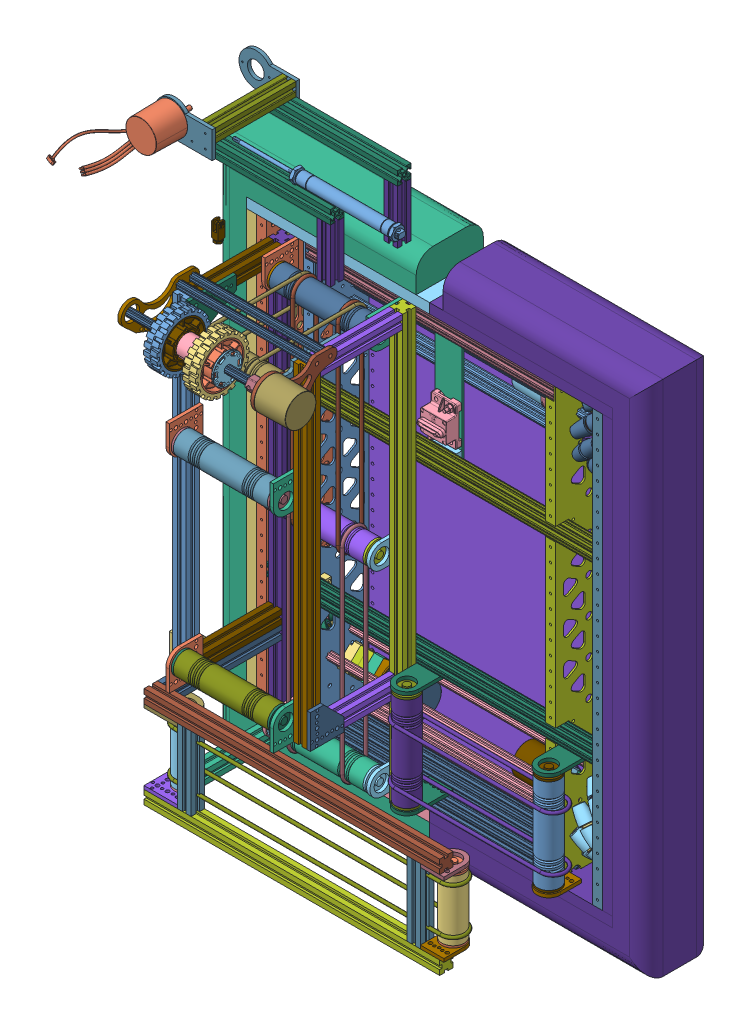
SolidWorks assembly Robot 2020, configuration Default. Lengths in mm. (continued)
Components (placement in the parent): (continued)
- Robot 2020(2)^Robot 2020-1: Robot 2020(2)^Robot 2020 [Default] at origin size (819.15 992.53 549) (virtual) (continued)
  - Snake^Robot 2020(2)_Robot 2020-1: Snake^Robot 2020(2)_Robot 2020 [Default] at (-279.4 -406.4 122.2875) x (0 -1 0) z (0 0 1) size (812.8 266.7 245.82) (virtual) (continued)
    - Longest Belt^Snake_Robot 2020(2)_Robot 2020-2: Longest Belt^Snake_Robot 2020(2)_Robot 2020 [Default] at (-411.1625 176.276 39.6875) size (421.79 6 50.31) (virtual)
    - Front Bearing Bracket^Snake_Robot 2020(2)_Robot 2020-1: Front Bearing Bracket^Snake_Robot 2020(2)_Robot 2020 [Default] at (-812.8 222.25 180.975) size (63.5 6.35 127) (virtual)
    - Front Bearing Bracket_1^Snake_Robot 2020(2)_Robot 2020-1: Front Bearing Bracket_1^Snake_Robot 2020(2)_Robot 2020 [Default] at (-812.8 25.4 180.975) size (63.5 6.35 127) (virtual)
  - Serializer^Robot 2020(2)_Robot 2020-1: Serializer^Robot 2020(2)_Robot 2020 [Default] at (-279.4 -406.4 96.8875) size (577.61 228.6 285.75) (virtual)
    - Roller_6^Serializer_Robot 2020(2)_Robot 2020-1: Roller_6^Serializer_Robot 2020(2)_Robot 2020 [Default] at origin size (42.07 200.15 42.07) (virtual)
      - Roller Hub^Roller_6_Serializer_Robot 2020(2)_Robot 2020-1: Roller Hub^Roller_6_Serializer_Robot 2020(2)_Robot 2020 [Default] at (276.225 31.75 65.0875) size (42.07 25.4 42.07) (virtual)
      - Roller 7^Roller_6_Serializer_Robot 2020(2)_Robot 2020-1: Roller 7^Roller_6_Serializer_Robot 2020(2)_Robot 2020 [Default] at (276.225 125.476 65.0875) size (42.07 177.8 42.07) (virtual)
      - Roller Hub^Roller_6_Serializer_Robot 2020(2)_Robot 2020-2: Roller Hub^Roller_6_Serializer_Robot 2020(2)_Robot 2020 [Default] at (276.225 219.202 65.0875) x (1 0 0) z (0 0 -1) size (42.07 25.4 42.07) (virtual)
    - Roller_7^Serializer_Robot 2020(2)_Robot 2020-1: Roller_7^Serializer_Robot 2020(2)_Robot 2020 [Default] at origin size (42.07 200.15 42.07) (virtual)
      - Roller Hub^Roller_7_Serializer_Robot 2020(2)_Robot 2020-1: Roller Hub^Roller_7_Serializer_Robot 2020(2)_Robot 2020 [Default] at (544.5125 31.75 65.0875) size (42.07 25.4 42.07) (virtual)
      - Roller 7^Roller_7_Serializer_Robot 2020(2)_Robot 2020-1: Roller 7^Roller_7_Serializer_Robot 2020(2)_Robot 2020 [Default] at (544.5125 125.476 65.0875) size (42.07 177.8 42.07) (virtual)
      - Roller Hub^Roller_7_Serializer_Robot 2020(2)_Robot 2020-2: Roller Hub^Roller_7_Serializer_Robot 2020(2)_Robot 2020 [Default] at (544.5125 219.202 65.0875) x (1 0 0) z (0 0 -1) size (42.07 25.4 42.07) (virtual)
    - Roller Short^Serializer_Robot 2020(2)_Robot 2020-1: Roller Short^Serializer_Robot 2020(2)_Robot 2020 [Default] at origin size (42.07 136.65 42.07) (virtual)
      - Roller Hub^Roller Short_Serializer_Robot 2020(2)_Robot 2020-1: Roller Hub^Roller Short_Serializer_Robot 2020(2)_Robot 2020 [Default] at (544.5125 31.75 246.0625) size (42.07 25.4 42.07) (virtual)
      - Roller 4.5^Roller Short_Serializer_Robot 2020(2)_Robot 2020-1: Roller 4.5^Roller Short_Serializer_Robot 2020(2)_Robot 2020 [Default] at (544.5125 93.726 246.0625) size (42.07 114.3 42.07) (virtual)
      - Roller Hub^Roller Short_Serializer_Robot 2020(2)_Robot 2020-2: Roller Hub^Roller Short_Serializer_Robot 2020(2)_Robot 2020 [Default] at (544.5125 155.702 246.0625) x (1 0 0) z (0 0 -1) size (42.07 25.4 42.07) (virtual)
    - Roller Short_1^Serializer_Robot 2020(2)_Robot 2020-1: Roller Short_1^Serializer_Robot 2020(2)_Robot 2020 [Default] at origin size (42.07 136.65 42.07) (virtual)
      - Roller Hub^Roller Short_1_Serializer_Robot 2020(2)_Robot 2020-1: Roller Hub^Roller Short_1_Serializer_Robot 2020(2)_Robot 2020 [Default] at (39.6875 31.75 246.0625) size (42.07 25.4 42.07) (virtual)
      - Roller 4.5^Roller Short_1_Serializer_Robot 2020(2)_Robot 2020-1: Roller 4.5^Roller Short_1_Serializer_Robot 2020(2)_Robot 2020 [Default] at (39.6875 93.726 246.0625) size (42.07 114.3 42.07) (virtual)
      - Roller Hub^Roller Short_1_Serializer_Robot 2020(2)_Robot 2020-2: Roller Hub^Roller Short_1_Serializer_Robot 2020(2)_Robot 2020 [Default] at (39.6875 155.702 246.0625) x (1 0 0) z (0 0 -1) size (42.07 25.4 42.07) (virtual)
    - 1010-8.25^Serializer_Robot 2020(2)_Robot 2020-1: 1010-8.25^Serializer_Robot 2020(2)_Robot 2020 [Default] at (12.7 12.7 50.8) size (25.4 25.4 209.55) (virtual)
    - 1010-22^Serializer_Robot 2020(2)_Robot 2020-1: 1010-22^Serializer_Robot 2020(2)_Robot 2020 [Default] at (0 12.7 273.05) x (0 0 -1) z (1 0 0) size (25.4 25.4 558.8) (virtual)
    - Corner Bearing Bracket^Serializer_Robot 2020(2)_Robot 2020-1: Corner Bearing Bracket^Serializer_Robot 2020(2)_Robot 2020 [Default] at (0 25.4 285.75) x (0 0 -1) z (1 0 0) size (63.5 6.35 63.5) (virtual)
    - Center Bearing Bracket^Serializer_Robot 2020(2)_Robot 2020-1: Center Bearing Bracket^Serializer_Robot 2020(2)_Robot 2020 [Default] at (522.2875 25.4 25.4) size (44.45 6.35 61.91) (virtual)
    - Center Bearing Bracket^Serializer_Robot 2020(2)_Robot 2020-2: Center Bearing Bracket^Serializer_Robot 2020(2)_Robot 2020 [Default] at (566.7375 25.4 285.75) x (-1 0 0) z (0 0 -1) size (44.45 6.35 61.91) (virtual)
    - 1010-8.25 v1(Mirror)^Serializer_Robot 2020(2)_Robot 2020-1: 1010-8.25 v1(Mirror)^Serializer_Robot 2020(2)_Robot 2020 [Default] at (12.7 177.8 50.8) x (1 0 0) z (0 0 -1) size (25.4 25.4 209.55) (virtual)
    - 1010-22 v1(Mirror)^Serializer_Robot 2020(2)_Robot 2020-1: 1010-22 v1(Mirror)^Serializer_Robot 2020(2)_Robot 2020 [Default] at (0 177.8 273.05) x (0 0 -1) z (-1 0 0) size (25.4 25.4 558.8) (virtual)
    - Corner Bearing Bracket v2(Mirror)^Serializer_Robot 2020(2)_Robot 2020-1: Corner Bearing Bracket v2(Mirror)^Serializer_Robot 2020(2)_Robot 2020 [Default] at (0 165.1 285.75) x (0 0 -1) z (-1 0 0) size (63.5 6.35 63.5) (virtual)
    - Center Bearing Bracket v3(Mirror)^Serializer_Robot 2020(2)_Robot 2020-1: Center Bearing Bracket v3(Mirror)^Serializer_Robot 2020(2)_Robot 2020 [Default] at (566.7375 165.1 285.75) x (-1 0 0) z (0 0 1) size (44.45 6.35 61.91) (virtual)
    - 1010-5.5^Serializer_Robot 2020(2)_Robot 2020-1: 1010-5.5^Serializer_Robot 2020(2)_Robot 2020 [Default] at (76.2 25.4 273.05) x (1 0 0) z (0 1 0) size (25.4 25.4 139.7) (virtual)
    - 1010-5.5^Serializer_Robot 2020(2)_Robot 2020-2: 1010-5.5^Serializer_Robot 2020(2)_Robot 2020 [Default] at (509.5875 165.1 273.05) x (1 0 0) z (0 -1 0) size (25.4 25.4 139.7) (virtual)
    - Center Bearing Bracket Tall^Serializer_Robot 2020(2)_Robot 2020-1: Center Bearing Bracket Tall^Serializer_Robot 2020(2)_Robot 2020 [Default] at (254 222.25 0) size (44.45 6.35 87.31) (virtual)
    - Center Bearing Bracket Tall^Serializer_Robot 2020(2)_Robot 2020-2: Center Bearing Bracket Tall^Serializer_Robot 2020(2)_Robot 2020 [Default] at (522.2875 222.25 0) size (44.45 6.35 87.31) (virtual)
    - Center Bearing Bracket Tall^Serializer_Robot 2020(2)_Robot 2020-3: Center Bearing Bracket Tall^Serializer_Robot 2020(2)_Robot 2020 [Default] at (254 25.4 0) size (44.45 6.35 87.31) (virtual)
    - Serializer Long Belt^Serializer_Robot 2020(2)_Robot 2020-1: Serializer Long Belt^Serializer_Robot 2020(2)_Robot 2020 [Default] at (39.6875 50.926 246.0625) size (555.14 6 50.31) (virtual)
    - Serializer Long Belt^Serializer_Robot 2020(2)_Robot 2020-2: Serializer Long Belt^Serializer_Robot 2020(2)_Robot 2020 [Default] at (39.6875 136.526 246.0625) size (555.14 6 50.31) (virtual)
    - Serializer Short Belt^Serializer_Robot 2020(2)_Robot 2020-1: Serializer Short Belt^Serializer_Robot 2020(2)_Robot 2020 [Default] at (276.225 66.676 65.0875) size (326.54 6 50.31) (virtual)
    - Serializer Short Belt^Serializer_Robot 2020(2)_Robot 2020-2: Serializer Short Belt^Serializer_Robot 2020(2)_Robot 2020 [Default] at (276.225 168.276 65.0875) size (326.54 6 50.31) (virtual)
  - Shooter Assembly^Robot 2020(2)_Robot 2020-1: Shooter Assembly^Robot 2020(2)_Robot 2020 [Default] at (-152.4 406.3995 328.6625) x (0 -1 0) z (0 0 1) size (189.59 325.45 222.03) (virtual)
    - Wheel Assembly^Shooter Assembly_Robot 2020(2)_Robot 2020-1: Wheel Assembly^Shooter Assembly_Robot 2020(2)_Robot 2020 [Default] at (-2.4561 -5.69 76.4329) x (0.5 0 0.866025) z (0 -1 0) size (138.79 138.79 119.38) (virtual)
      - am-2256 HiGrip Wheel-1: am-2256 HiGrip Wheel [Default] at (-0.933 3.4526 44.5642) x (0 0 1) z (0.866025 -0.5 0) size (35.12 101.6 101.6)
        - 4in 2013 Hub^am-2256 HiGrip Wheel-1: 4in 2013 Hub^am-2256 HiGrip Wheel [Default] at (-8.0517 2.5236 2.5343) size (35.12 82.55 82.55) (virtual)
        - 4 in tread^am-2256 HiGrip Wheel-1: 4 in tread^am-2256 HiGrip Wheel [Default] at (-8.0517 2.5236 2.5343) size (25.4 101.6 101.6) (virtual)
      - am-2256 4 in HiGrip Wheel_1^Wheel Assembly_Shooter Assembly_Robot 2020(2)_Robot 2020-1: am-2256 4 in HiGrip Wheel_1^Wheel Assembly_Shooter Assembly_Robot 2020(2)_Robot 2020 [Default] at (-3.4565 0.9183 -28.4608) x (0 0 1) z (0.866025 0.5 0) size (35.12 101.6 101.6) (virtual)
        - 4in 2013 Hub^am-2256 4 in HiGrip Wheel_1_Wheel Assembly_Shooter Assembly_Robot 2020(2)_Robot 2020-1: 4in 2013 Hub^am-2256 4 in HiGrip Wheel_1_Wheel Assembly_Shooter Assembly_Robot 2020(2)_Robot 2020 [Default] at (-8.0517 2.5236 2.5343) size (35.12 82.55 82.55) (virtual)
        - 4 in tread^am-2256 4 in HiGrip Wheel_1_Wheel Assembly_Shooter Assembly_Robot 2020(2)_Robot 2020-1: 4 in tread^am-2256 4 in HiGrip Wheel_1_Wheel Assembly_Shooter Assembly_Robot 2020(2)_Robot 2020 [Default] at (-8.0517 2.5236 2.5343) size (25.4 101.6 101.6) (virtual)
      - Wheel Center Spacer^Wheel Assembly_Shooter Assembly_Robot 2020(2)_Robot 2020-1: Wheel Center Spacer^Wheel Assembly_Shooter Assembly_Robot 2020(2)_Robot 2020 [Default] at origin size (37.36 38.1 50.8) (virtual)
      - 1_2_Hex_Bore_Aluminum_Versa Hub-1: 1_2_Hex_Bore_Aluminum_Versa Hub [Default] at (0 0 -46.99) x (0 0 -1) z (0.866025 0.5 0) size (12.7 55.88 55.88)
      - 1_2_Hex_Bore_Aluminum_VersaHub_217-2592 v1(Mirror)_1^Wheel Assembly_Shooter Assembly_Robot 2020(2)_Robot 2020-1: 1_2_Hex_Bore_Aluminum_VersaHub_217-2592 v1(Mirror)_1^Wheel Assembly_Shooter Assembly_Robot 2020(2)_Robot 2020 [Default] at (0 0 46.99) x (0 0 1) z (-0.866025 -0.5 0) size (12.7 55.88 55.88) (virtual)
    - Frame Bottom Pivot^Shooter Assembly_Robot 2020(2)_Robot 2020-1: Frame Bottom Pivot^Shooter Assembly_Robot 2020(2)_Robot 2020 [Default] at (57.6875 -114.3 11.2014) size (49 22.4 25.4) (virtual)
    - Frame Bottom Pivot v1(Mirror)^Shooter Assembly_Robot 2020(2)_Robot 2020-1: Frame Bottom Pivot v1(Mirror)^Shooter Assembly_Robot 2020(2)_Robot 2020 [Default] at (57.6875 114.3 11.2014) x (1 0 0) z (0 0 -1) size (49 22.4 25.4) (virtual)
    - Bottom Frame Bearing Side^Shooter Assembly_Robot 2020(2)_Robot 2020-1: Bottom Frame Bearing Side^Shooter Assembly_Robot 2020(2)_Robot 2020 [Default] at (39.6875 -133.35 14.2875) size (75.84 6.35 148.23) (virtual)
    - Churro 10_^Shooter Assembly_Robot 2020(2)_Robot 2020-1: Churro 10_^Shooter Assembly_Robot 2020(2)_Robot 2020 [Default] at (-6.35 177.8 -12.7) x (1 0 0) z (0 -1 0) size (14.66 12.7 254) (virtual)
    - Churro 10_^Shooter Assembly_Robot 2020(2)_Robot 2020-2: Churro 10_^Shooter Assembly_Robot 2020(2)_Robot 2020 [Default] at (-6.35 177.8 -38.1) x (1 0 0) z (0 -1 0) size (14.66 12.7 254) (virtual)
    - Bottom Frame Motor Side^Shooter Assembly_Robot 2020(2)_Robot 2020-1: Bottom Frame Motor Side^Shooter Assembly_Robot 2020(2)_Robot 2020 [Default] at (39.6875 127 14.2875) size (84.84 6.35 157.23) (virtual)
    - NEO Motor REV-21-1650^Shooter Assembly_Robot 2020(2)_Robot 2020-1: NEO Motor REV-21-1650^Shooter Assembly_Robot 2020(2)_Robot 2020 [Default] at (-2.4561 133.35 76.4329) x (-1 0 0) z (0 -1 0) size (61.14 61.02 93.25) (virtual)
    - Motor to Hex Adapter^Shooter Assembly_Robot 2020(2)_Robot 2020-1: Motor to Hex Adapter^Shooter Assembly_Robot 2020(2)_Robot 2020 [Default] at (-2.4561 123.85 76.4329) x (0 0 -1) z (0 -1 0) size (24.79 22 25.4) (virtual)
    - Churro 10_^Shooter Assembly_Robot 2020(2)_Robot 2020-3: Churro 10_^Shooter Assembly_Robot 2020(2)_Robot 2020 [Default] at (-2.4561 170.95 76.4329) x (0.866025 0 0.5) z (0 -1 0) size (14.66 12.7 254) (virtual)
- LiftingThing-1: LiftingThing [Default] at (-286.0132 645.5427 249.3316) size (485.32 165.1 334.88)
  - MotorMount-1: MotorMount [Default] at (21.5971 61.1717 89.4409) size (107.95 63.5 6.35)
  - supportBar-1: supportBar [Default] at (314.868 42.1217 76.7409) x (0 0 -1) z (1 0 0) size (25.4 25.4 254)
  - horrizontalBar-1: horrizontalBar [Default] at (85.0971 67.5217 89.4409) size (25.4 25.4 152.4)
  - MotorMount-2: MotorMount [Default] at (21.5971 61.1717 -69.3091) size (107.95 63.5 6.35)
  - supportBar-2: supportBar [Default] at (60.868 42.1217 -50.2591) x (0 1 0) z (-1 0 0) size (25.4 25.4 254)
  - HingeMount-1: HingeMount [Default] at (302.168 29.4217 76.7409) x (1 0 0) z (0 1 0) size (25.4 25.4 101.6)
  - HingeMount-2: HingeMount [Default] at (302.168 29.4217 -50.2591) x (1 0 0) z (0 1 0) size (25.4 25.4 101.6)
  - 6498K420_ROUND BODY AIR CYLINDER-1: 6498K420_ROUND BODY AIR CYLINDER [6498K42] at (144.6448 -56.0854 131.2964) size (17.53 35.92 12.7)
  - 6498K636_ROUND BODY AIR CYLINDER-1: 6498K636_ROUND BODY AIR CYLINDER [6498K636] at (329.4526 67.6458 76.6686) x (1 0 0) z (0 -0.999962 0.008727) size (318.84 27.5 23.81)
  - NEO_REV-21-1650-1: NEO_REV-21-1650 [Default] at (21.5971 61.1717 95.7909) x (1 0 0) z (0 0 -1) size (98.87 73.45 204.78)
